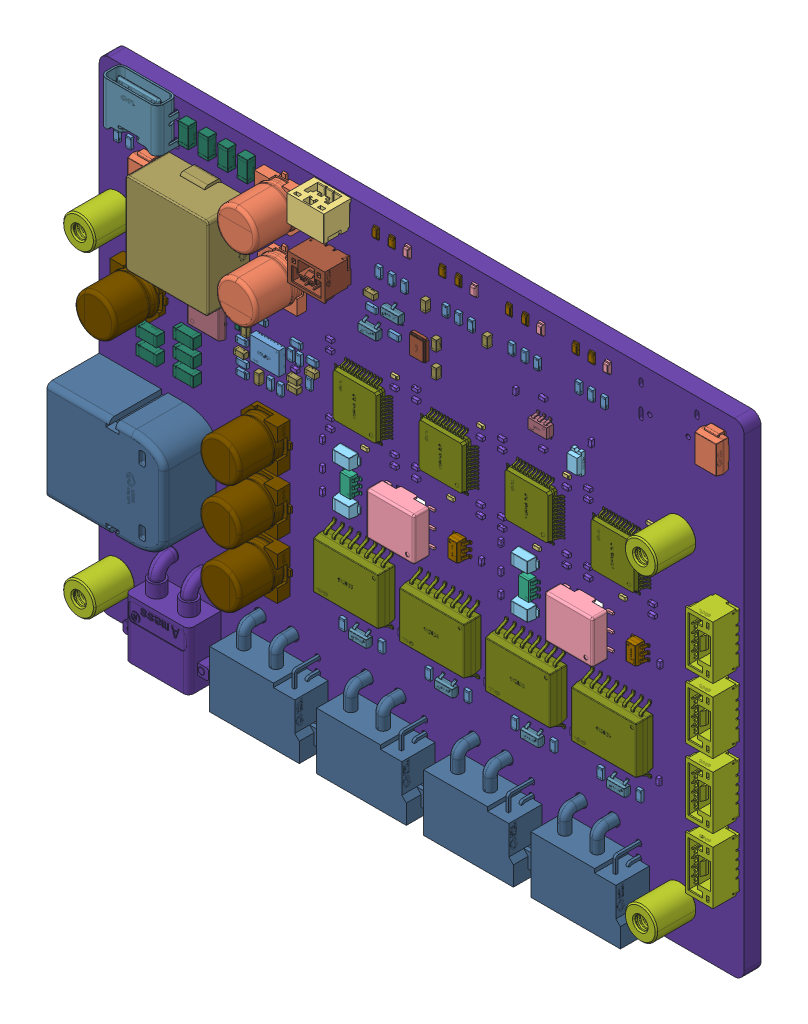
SolidWorks assembly 三合一(1), configuration 默认. Lengths in mm.
Overall size (99.98 75.08 11.76).
370 component instances, 35 part files, 0 mates.
Components (placement in the parent):
- 三合一(1).step-1: 三合一(1).step [默认] at origin size (99.98 75.08 11.76)
  - R75~R0603~R0603~5cPJ.step-1: R75~R0603~R0603~5cPJ.step [默认] at (-28.5751 -8.895 -0.01) x (0 -1 0) z (0 0 -1) size (0.81 1.62 0.45)
    - R0603~R0603~Wemx.step-1: R0603~R0603~Wemx.step [默认] at origin size (0.81 1.62 0.45)
  - R159~R0603~R0603~W8s1.step-1: R159~R0603~R0603~W8s1.step [默认] at (-17.4062 29.8554 2.6401) x (-1 0 0) z (0 0 1) size (0.81 1.62 0.45)
    - R0603~R0603~Wemx.step-1: R0603~R0603~Wemx.step [默认] at origin size (0.81 1.62 0.45)
  - R160~R0603~R0603~Jkel.step-1: R160~R0603~R0603~Jkel.step [默认] at (-15.4326 29.8554 2.6401) x (-1 0 0) z (0 0 1) size (0.81 1.62 0.45)
    - R0603~R0603~Wemx.step-1: R0603~R0603~Wemx.step [默认] at origin size (0.81 1.62 0.45)
  - R164~R0603~R0603~qJS6.step-1: R164~R0603~R0603~qJS6.step [默认] at (-13.459 29.8554 2.6401) x (-1 0 0) z (0 0 1) size (0.81 1.62 0.45)
    - R0603~R0603~Wemx.step-1: R0603~R0603~Wemx.step [默认] at origin size (0.81 1.62 0.45)
  - R165~R0603~R0603~esAK.step-1: R165~R0603~R0603~esAK.step [默认] at (-7.0403 29.8554 2.6401) x (-1 0 0) z (0 0 1) size (0.81 1.62 0.45)
    - R0603~R0603~Wemx.step-1: R0603~R0603~Wemx.step [默认] at origin size (0.81 1.62 0.45)
  - R166~R0603~R0603~Am0v.step-1: R166~R0603~R0603~Am0v.step [默认] at (-5.0667 29.8554 2.6401) x (-1 0 0) z (0 0 1) size (0.81 1.62 0.45)
    - R0603~R0603~Wemx.step-1: R0603~R0603~Wemx.step [默认] at origin size (0.81 1.62 0.45)
  - R167~R0603~R0603~RGyW.step-1: R167~R0603~R0603~RGyW.step [默认] at (-3.0931 29.8554 2.6401) x (-1 0 0) z (0 0 1) size (0.81 1.62 0.45)
    - R0603~R0603~Wemx.step-1: R0603~R0603~Wemx.step [默认] at origin size (0.81 1.62 0.45)
  - R168~R0603~R0603~ARsL.step-1: R168~R0603~R0603~ARsL.step [默认] at (3.1985 29.8554 2.6401) x (-1 0 0) z (0 0 1) size (0.81 1.62 0.45)
    - R0603~R0603~Wemx.step-1: R0603~R0603~Wemx.step [默认] at origin size (0.81 1.62 0.45)
  - R169~R0603~R0603~JQ4Y.step-1: R169~R0603~R0603~JQ4Y.step [默认] at (5.1721 29.8554 2.6401) x (-1 0 0) z (0 0 1) size (0.81 1.62 0.45)
    - R0603~R0603~Wemx.step-1: R0603~R0603~Wemx.step [默认] at origin size (0.81 1.62 0.45)
  - R170~R0603~R0603~c30l.step-1: R170~R0603~R0603~c30l.step [默认] at (7.1457 29.8554 2.6401) x (-1 0 0) z (0 0 1) size (0.81 1.62 0.45)
    - R0603~R0603~Wemx.step-1: R0603~R0603~Wemx.step [默认] at origin size (0.81 1.62 0.45)
  - R171~R0603~R0603~cDsC.step-1: R171~R0603~R0603~cDsC.step [默认] at (13.5643 29.8554 2.6401) x (-1 0 0) z (0 0 1) size (0.81 1.62 0.45)
    - R0603~R0603~Wemx.step-1: R0603~R0603~Wemx.step [默认] at origin size (0.81 1.62 0.45)
  - R172~R0603~R0603~ldmr.step-1: R172~R0603~R0603~ldmr.step [默认] at (15.5379 29.8554 2.6401) x (-1 0 0) z (0 0 1) size (0.81 1.62 0.45)
    - R0603~R0603~Wemx.step-1: R0603~R0603~Wemx.step [默认] at origin size (0.81 1.62 0.45)
  - R173~R0603~R0603~DBhJ.step-1: R173~R0603~R0603~DBhJ.step [默认] at (17.5115 29.8554 2.6401) x (-1 0 0) z (0 0 1) size (0.81 1.62 0.45)
    - R0603~R0603~Wemx.step-1: R0603~R0603~Wemx.step [默认] at origin size (0.81 1.62 0.45)
  - R151~R0603~R0603~Tuse.step-1: R151~R0603~R0603~Tuse.step [默认] at (-18.516 24.4061 2.6401) x (0 -1 0) z (0 0 1) size (0.81 1.62 0.45)
    - R0603~R0603~Wemx.step-1: R0603~R0603~Wemx.step [默认] at origin size (0.81 1.62 0.45)
  - R137~R0603~R0603~KOhT.step-1: R137~R0603~R0603~KOhT.step [默认] at (-22.995 -20.1855 2.6401) size (0.81 1.62 0.45)
    - R0603~R0603~Wemx.step-1: R0603~R0603~Wemx.step [默认] at origin size (0.81 1.62 0.45)
  - R152~R0603~R0603~idg1.step-1: R152~R0603~R0603~idg1.step [默认] at (-15.016 22.484 2.6401) x (0 1 0) z (0 0 1) size (0.81 1.62 0.45)
    - R0603~R0603~Wemx.step-1: R0603~R0603~Wemx.step [默认] at origin size (0.81 1.62 0.45)
  - CS6~R0603~R0603~lHR4.step-1: CS6~R0603~R0603~lHR4.step [默认] at (23.005 -20.1855 2.6401) size (0.81 1.62 0.45)
    - R0603~R0603~Wemx.step-1: R0603~R0603~Wemx.step [默认] at origin size (0.81 1.62 0.45)
  - R141~R0603~R0603~uq1I.step-1: R141~R0603~R0603~uq1I.step [默认] at (-9.6617 -20.1855 2.6401) size (0.81 1.62 0.45)
    - R0603~R0603~Wemx.step-1: R0603~R0603~Wemx.step [默认] at origin size (0.81 1.62 0.45)
  - CS5~R0603~R0603~782x.step-1: CS5~R0603~R0603~782x.step [默认] at (9.6717 -20.1855 2.6401) size (0.81 1.62 0.45)
    - R0603~R0603~Wemx.step-1: R0603~R0603~Wemx.step [默认] at origin size (0.81 1.62 0.45)
  - R144~R0603~R0603~EvhU.step-1: R144~R0603~R0603~EvhU.step [默认] at (3.6717 -20.1855 2.6401) size (0.81 1.62 0.45)
    - R0603~R0603~Wemx.step-1: R0603~R0603~Wemx.step [默认] at origin size (0.81 1.62 0.45)
  - CS7~R0603~R0603~eEbJ.step-1: CS7~R0603~R0603~eEbJ.step [默认] at (-3.6617 -20.1855 2.6401) size (0.81 1.62 0.45)
    - R0603~R0603~Wemx.step-1: R0603~R0603~Wemx.step [默认] at origin size (0.81 1.62 0.45)
  - R147~R0603~R0603~I41l.step-1: R147~R0603~R0603~I41l.step [默认] at (17.005 -20.1855 2.6401) size (0.81 1.62 0.45)
    - R0603~R0603~Wemx.step-1: R0603~R0603~Wemx.step [默认] at origin size (0.81 1.62 0.45)
  - CS8~R0603~R0603~DkA6.step-1: CS8~R0603~R0603~DkA6.step [默认] at (-16.995 -20.1855 2.6401) size (0.81 1.62 0.45)
    - R0603~R0603~Wemx.step-1: R0603~R0603~Wemx.step [默认] at origin size (0.81 1.62 0.45)
  - R1~R0402~R0603~QKKM.step-1: R1~R0402~R0603~QKKM.step [默认] at (-29.788 11.9413 2.6401) x (-1 0 0) z (0 0 1) size (0.81 1.62 0.45)
    - R0603~R0603~Wemx.step-1: R0603~R0603~Wemx.step [默认] at origin size (0.81 1.62 0.45)
  - R2~R0402~R0603~ICsz.step-1: R2~R0402~R0603~ICsz.step [默认] at (-31.0503 11.9335 2.6401) size (0.81 1.62 0.45)
    - R0603~R0603~Wemx.step-1: R0603~R0603~Wemx.step [默认] at origin size (0.81 1.62 0.45)
  - R3~R0402~R0603~sk96.step-1: R3~R0402~R0603~sk96.step [默认] at (-32.6863 6.4398 2.6401) size (0.81 1.62 0.45)
    - R0603~R0603~Wemx.step-1: R0603~R0603~Wemx.step [默认] at origin size (0.81 1.62 0.45)
  - R4~R0402~R0603~okoP.step-1: R4~R0402~R0603~okoP.step [默认] at (-38.5703 5.6081 2.6401) x (0 -1 0) z (0 0 1) size (0.81 1.62 0.45)
    - R0603~R0603~Wemx.step-1: R0603~R0603~Wemx.step [默认] at origin size (0.81 1.62 0.45)
  - R5~R0402~R0603~vXkP.step-1: R5~R0402~R0603~vXkP.step [默认] at (-34.283 6.4398 2.6401) x (-1 0 0) z (0 0 1) size (0.81 1.62 0.45)
    - R0603~R0603~Wemx.step-1: R0603~R0603~Wemx.step [默认] at origin size (0.81 1.62 0.45)
  - R6~R0402~R0603~4bc1.step-1: R6~R0402~R0603~4bc1.step [默认] at (-28.1899 9.4911 2.6401) size (0.81 1.62 0.45)
    - R0603~R0603~Wemx.step-1: R0603~R0603~Wemx.step [默认] at origin size (0.81 1.62 0.45)
  - R7~R0402~R0603~K2X5.step-1: R7~R0402~R0603~K2X5.step [默认] at (-27.7516 12.6103 2.6401) x (0 -1 0) z (0 0 1) size (0.81 1.62 0.45)
    - R0603~R0603~Wemx.step-1: R0603~R0603~Wemx.step [默认] at origin size (0.81 1.62 0.45)
  - R8~R0402~R0603~ww3o.step-1: R8~R0402~R0603~ww3o.step [默认] at (-38.5577 7.046 2.6401) x (0 1 0) z (0 0 1) size (0.81 1.62 0.45)
    - R0603~R0603~Wemx.step-1: R0603~R0603~Wemx.step [默认] at origin size (0.81 1.62 0.45)
  - R9~R0402~R0603~rL22.step-1: R9~R0402~R0603~rL22.step [默认] at (-47.1895 9.6666 -0.01) x (-1 0 0) z (0 0 -1) size (0.81 1.62 0.45)
    - R0603~R0603~Wemx.step-1: R0603~R0603~Wemx.step [默认] at origin size (0.81 1.62 0.45)
  - R10~R0402~R0603~MKr8.step-1: R10~R0402~R0603~MKr8.step [默认] at (-30.2287 13.7786 2.6401) x (0 -1 0) z (0 0 1) size (0.81 1.62 0.45)
    - R0603~R0603~Wemx.step-1: R0603~R0603~Wemx.step [默认] at origin size (0.81 1.62 0.45)
  - R11~R0402~R0603~NHCh.step-1: R11~R0402~R0603~NHCh.step [默认] at (-35.6203 16.6165 2.6401) x (0 -1 0) z (0 0 1) size (0.81 1.62 0.45)
    - R0603~R0603~Wemx.step-1: R0603~R0603~Wemx.step [默认] at origin size (0.81 1.62 0.45)
  - R12~R0402~R0603~EJ67.step-1: R12~R0402~R0603~EJ67.step [默认] at (-35.62 15.4211 2.6401) x (0 1 0) z (0 0 1) size (0.81 1.62 0.45)
    - R0603~R0603~Wemx.step-1: R0603~R0603~Wemx.step [默认] at origin size (0.81 1.62 0.45)
  - R13~R0402~R0603~bliZ.step-1: R13~R0402~R0603~bliZ.step [默认] at (-35.6223 14.1624 2.6401) x (0 -1 0) z (0 0 1) size (0.81 1.62 0.45)
    - R0603~R0603~Wemx.step-1: R0603~R0603~Wemx.step [默认] at origin size (0.81 1.62 0.45)
  - R14~R0402~R0603~ipD6.step-1: R14~R0402~R0603~ipD6.step [默认] at (-38.6391 9.9522 2.6401) x (0 -1 0) z (0 0 1) size (0.81 1.62 0.45)
    - R0603~R0603~Wemx.step-1: R0603~R0603~Wemx.step [默认] at origin size (0.81 1.62 0.45)
  - R15~R0402~R0603~8ieX.step-1: R15~R0402~R0603~8ieX.step [默认] at (-28.8291 -15.616 -0.01) x (0 1 0) z (0 0 -1) size (0.81 1.62 0.45)
    - R0603~R0603~Wemx.step-1: R0603~R0603~Wemx.step [默认] at origin size (0.81 1.62 0.45)
  - R133~R0603~R0603~qmoj.step-1: R133~R0603~R0603~qmoj.step [默认] at (-56.0797 27.9566 2.6401) x (-1 0 0) z (0 0 1) size (0.81 1.62 0.45)
    - R0603~R0603~Wemx.step-1: R0603~R0603~Wemx.step [默认] at origin size (0.81 1.62 0.45)
  - R134~R0603~R0603~4lHX.step-1: R134~R0603~R0603~4lHX.step [默认] at (-57.9847 27.9566 2.6401) x (-1 0 0) z (0 0 1) size (0.81 1.62 0.45)
    - R0603~R0603~Wemx.step-1: R0603~R0603~Wemx.step [默认] at origin size (0.81 1.62 0.45)
  - D16~SMB_L4.6-W3.6-LS5.3-BI~SMB_L4.6-W3.6-LS5.3-BI~ZBYy.step-1: D16~SMB_L4.6-W3.6-LS5.3-BI~SMB_L4.6-W3.6-LS5.3-BI~ZBYy.step [默认] at (-52.8886 25.4111 2.7301) x (0 1 0) z (0 0 1) size (5.4 3.6 2.1)
    - SMB_L4.6-W3.6-LS5.3-BI~SMB_L4.6-W3.6-LS5.3-BI~m2hS.step-1: SMB_L4.6-W3.6-LS5.3-BI~SMB_L4.6-W3.6-LS5.3-BI~m2hS.step [默认] at origin size (5.4 3.6 2.1)
  - D15~SMB_L4.6-W3.6-LS5.3-BI~SMB_L4.6-W3.6-LS5.3-BI~mUhA.step-1: D15~SMB_L4.6-W3.6-LS5.3-BI~SMB_L4.6-W3.6-LS5.3-BI~mUhA.step [默认] at (35.0521 32.5121 2.7301) x (0 -1 0) z (0 0 1) size (5.4 3.6 2.1)
    - SMB_L4.6-W3.6-LS5.3-BI~SMB_L4.6-W3.6-LS5.3-BI~m2hS.step-1: SMB_L4.6-W3.6-LS5.3-BI~SMB_L4.6-W3.6-LS5.3-BI~m2hS.step [默认] at origin size (5.4 3.6 2.1)
  - R136~R0402~R0402_L1.0-W0.5-H0.4~lcg2.step-1: R136~R0402~R0402_L1.0-W0.5-H0.4~lcg2.step [默认] at (-19.6434 5 2.6301) size (1 0.5 0.36)
    - R0402~R0402_L1.0-W0.5-H0.4~H1Nt.step-1: R0402~R0402_L1.0-W0.5-H0.4~H1Nt.step [默认] at origin size (1 0.5 0.36)
  - R135~R0402~R0402_L1.0-W0.5-H0.4~7DHQ.step-1: R135~R0402~R0402_L1.0-W0.5-H0.4~7DHQ.step [默认] at (-15 17 2.6301) x (-1 0 0) z (0 0 1) size (1 0.5 0.36)
    - R0402~R0402_L1.0-W0.5-H0.4~H1Nt.step-1: R0402~R0402_L1.0-W0.5-H0.4~H1Nt.step [默认] at origin size (1 0.5 0.36)
  - R140~R0402~R0402_L1.0-W0.5-H0.4~fAPd.step-1: R140~R0402~R0402_L1.0-W0.5-H0.4~fAPd.step [默认] at (-6.3101 5 2.6301) size (1 0.5 0.36)
    - R0402~R0402_L1.0-W0.5-H0.4~H1Nt.step-1: R0402~R0402_L1.0-W0.5-H0.4~H1Nt.step [默认] at origin size (1 0.5 0.36)
  - R139~R0402~R0402_L1.0-W0.5-H0.4~Vtb0.step-1: R139~R0402~R0402_L1.0-W0.5-H0.4~Vtb0.step [默认] at (-1.6667 17 2.6301) x (-1 0 0) z (0 0 1) size (1 0.5 0.36)
    - R0402~R0402_L1.0-W0.5-H0.4~H1Nt.step-1: R0402~R0402_L1.0-W0.5-H0.4~H1Nt.step [默认] at origin size (1 0.5 0.36)
  - R143~R0402~R0402_L1.0-W0.5-H0.4~u8e5.step-1: R143~R0402~R0402_L1.0-W0.5-H0.4~u8e5.step [默认] at (7.0233 5 2.6301) size (1 0.5 0.36)
    - R0402~R0402_L1.0-W0.5-H0.4~H1Nt.step-1: R0402~R0402_L1.0-W0.5-H0.4~H1Nt.step [默认] at origin size (1 0.5 0.36)
  - R142~R0402~R0402_L1.0-W0.5-H0.4~lItk.step-1: R142~R0402~R0402_L1.0-W0.5-H0.4~lItk.step [默认] at (11.6667 17 2.6301) x (-1 0 0) z (0 0 1) size (1 0.5 0.36)
    - R0402~R0402_L1.0-W0.5-H0.4~H1Nt.step-1: R0402~R0402_L1.0-W0.5-H0.4~H1Nt.step [默认] at origin size (1 0.5 0.36)
  - R146~R0402~R0402_L1.0-W0.5-H0.4~vA6z.step-1: R146~R0402~R0402_L1.0-W0.5-H0.4~vA6z.step [默认] at (20.3567 5 2.6301) size (1 0.5 0.36)
    - R0402~R0402_L1.0-W0.5-H0.4~H1Nt.step-1: R0402~R0402_L1.0-W0.5-H0.4~H1Nt.step [默认] at origin size (1 0.5 0.36)
  - R145~R0402~R0402_L1.0-W0.5-H0.4~Remo.step-1: R145~R0402~R0402_L1.0-W0.5-H0.4~Remo.step [默认] at (24.6191 17 2.6301) x (-1 0 0) z (0 0 1) size (1 0.5 0.36)
    - R0402~R0402_L1.0-W0.5-H0.4~H1Nt.step-1: R0402~R0402_L1.0-W0.5-H0.4~H1Nt.step [默认] at origin size (1 0.5 0.36)
  - LED18~LED0603-R-RD_GREEN~LED0603-RD_GREEN~kkZH.step-1: LED18~LED0603-R-RD_GREEN~LED0603-RD_GREEN~kkZH.step [默认] at (-13 34.7338 2.6401) x (0 -1 0) z (0 0 1) size (1.62 0.8 0.6)
    - LED0603-R-RD_GREEN~LED0603-RD_GREEN~Eb2N.step-1: LED0603-R-RD_GREEN~LED0603-RD_GREEN~Eb2N.step [默认] at origin size (1.62 0.8 0.6)
  - LED21~LED0603-R-RD_GREEN~LED0603-RD_GREEN~Mnfx.step-1: LED21~LED0603-R-RD_GREEN~LED0603-RD_GREEN~Mnfx.step [默认] at (-2.6667 34.76 2.6401) x (0 -1 0) z (0 0 1) size (1.62 0.8 0.6)
    - LED0603-R-RD_GREEN~LED0603-RD_GREEN~Eb2N.step-1: LED0603-R-RD_GREEN~LED0603-RD_GREEN~Eb2N.step [默认] at origin size (1.62 0.8 0.6)
  - LED24~LED0603-R-RD_GREEN~LED0603-RD_GREEN~tHpw.step-1: LED24~LED0603-R-RD_GREEN~LED0603-RD_GREEN~tHpw.step [默认] at (7.6667 34.7338 2.6401) x (0 -1 0) z (0 0 1) size (1.62 0.8 0.6)
    - LED0603-R-RD_GREEN~LED0603-RD_GREEN~Eb2N.step-1: LED0603-R-RD_GREEN~LED0603-RD_GREEN~Eb2N.step [默认] at origin size (1.62 0.8 0.6)
  - LED27~LED0603-R-RD_GREEN~LED0603-RD_GREEN~rwUx.step-1: LED27~LED0603-R-RD_GREEN~LED0603-RD_GREEN~rwUx.step [默认] at (18 34.7338 2.6401) x (0 -1 0) z (0 0 1) size (1.62 0.8 0.6)
    - LED0603-R-RD_GREEN~LED0603-RD_GREEN~Eb2N.step-1: LED0603-R-RD_GREEN~LED0603-RD_GREEN~Eb2N.step [默认] at origin size (1.62 0.8 0.6)
  - U107~SOD-123FL_L2.8-W1.9-LS3.7-RD~SOD-123FL_L2.8-W1.9-LS3.7-RD~TyNM.step-1: U107~SOD-123FL_L2.8-W1.9-LS3.7-RD~SOD-123FL_L2.8-W1.9-LS3.7-RD~TyNM.step [默认] at (5.4499 -3.754 2.8301) size (3.6 1.9 1.4)
    - SOD-123FL_L2.8-W1.9-LS3.7-RD~SOD-123FL_L2.8-W1.9-LS3.7-RD~L6eT.step-1: SOD-123FL_L2.8-W1.9-LS3.7-RD~SOD-123FL_L2.8-W1.9-LS3.7-RD~L6eT.step [默认] at origin size (3.6 1.9 1.4)
  - U22~SOD-123FL_L2.8-W1.9-LS3.7-RD~SOD-123FL_L2.8-W1.9-LS3.7-RD~IxVu.step-1: U22~SOD-123FL_L2.8-W1.9-LS3.7-RD~SOD-123FL_L2.8-W1.9-LS3.7-RD~IxVu.step [默认] at (5.4499 2.738 2.8301) size (3.6 1.9 1.4)
    - SOD-123FL_L2.8-W1.9-LS3.7-RD~SOD-123FL_L2.8-W1.9-LS3.7-RD~L6eT.step-1: SOD-123FL_L2.8-W1.9-LS3.7-RD~SOD-123FL_L2.8-W1.9-LS3.7-RD~L6eT.step [默认] at origin size (3.6 1.9 1.4)
  - U108~SOD-123FL_L2.8-W1.9-LS3.7-RD~SOD-123FL_L2.8-W1.9-LS3.7-RD~fh98.step-1: U108~SOD-123FL_L2.8-W1.9-LS3.7-RD~SOD-123FL_L2.8-W1.9-LS3.7-RD~fh98.step [默认] at (-22.212 -3.754 2.8301) size (3.6 1.9 1.4)
    - SOD-123FL_L2.8-W1.9-LS3.7-RD~SOD-123FL_L2.8-W1.9-LS3.7-RD~L6eT.step-1: SOD-123FL_L2.8-W1.9-LS3.7-RD~SOD-123FL_L2.8-W1.9-LS3.7-RD~L6eT.step [默认] at origin size (3.6 1.9 1.4)
  - U109~SOD-123FL_L2.8-W1.9-LS3.7-RD~SOD-123FL_L2.8-W1.9-LS3.7-RD~XY9i.step-1: U109~SOD-123FL_L2.8-W1.9-LS3.7-RD~SOD-123FL_L2.8-W1.9-LS3.7-RD~XY9i.step [默认] at (-22.212 2.738 2.8301) size (3.6 1.9 1.4)
    - SOD-123FL_L2.8-W1.9-LS3.7-RD~SOD-123FL_L2.8-W1.9-LS3.7-RD~L6eT.step-1: SOD-123FL_L2.8-W1.9-LS3.7-RD~SOD-123FL_L2.8-W1.9-LS3.7-RD~L6eT.step [默认] at origin size (3.6 1.9 1.4)
  - U24~SOT-23-5_L3.0-W1.6-P0.95-LS2.8-BR~SOT-23-5_L3.0-W1.6-P0.95-LS2.8-BR~zeFX.step-1: U24~SOT-23-5_L3.0-W1.6-P0.95-LS2.8-BR~SOT-23-5_L3.0-W1.6-P0.95-LS2.8-BR~zeFX.step [默认] at (6.0001 -0.508 3.5801) size (2.8 2.95 1.25)
    - SOT-23-5_L3.0-W1.6-P0.95-LS2.8-BR~SOT-23-5_L3.0-W1.6-P0.95-LS2.8-BR~bKoc.step-1: SOT-23-5_L3.0-W1.6-P0.95-LS2.8-BR~SOT-23-5_L3.0-W1.6-P0.95-LS2.8-BR~bKoc.step [默认] at origin size (2.8 2.95 1.25)
  - U110~SOT-23-5_L3.0-W1.6-P0.95-LS2.8-BR~SOT-23-5_L3.0-W1.6-P0.95-LS2.8-BR~mHFY.step-1: U110~SOT-23-5_L3.0-W1.6-P0.95-LS2.8-BR~SOT-23-5_L3.0-W1.6-P0.95-LS2.8-BR~mHFY.step [默认] at (-21.662 -0.508 3.5801) size (2.8 2.95 1.25)
    - SOT-23-5_L3.0-W1.6-P0.95-LS2.8-BR~SOT-23-5_L3.0-W1.6-P0.95-LS2.8-BR~bKoc.step-1: SOT-23-5_L3.0-W1.6-P0.95-LS2.8-BR~SOT-23-5_L3.0-W1.6-P0.95-LS2.8-BR~bKoc.step [默认] at origin size (2.8 2.95 1.25)
  - U7~SMD_BD5.0-D3.0~SMD_BD5.0-D3.0~2Aaa.step-1: U7~SMD_BD5.0-D3.0~SMD_BD5.0-D3.0~2Aaa.step [默认] at (-57.9392 17.87 1.2301) size (5 5 7.7)
    - SMD_BD5.0-D3.0~SMD_BD5.0-D3.0~7cq1.step-1: SMD_BD5.0-D3.0~SMD_BD5.0-D3.0~7cq1.step [默认] at origin size (5 5 7.7)
  - U8~SMD_BD5.0-D3.0~SMD_BD5.0-D3.0~8QZh.step-1: U8~SMD_BD5.0-D3.0~SMD_BD5.0-D3.0~8QZh.step [默认] at (29.1449 17.87 1.2301) size (5 5 7.7)
    - SMD_BD5.0-D3.0~SMD_BD5.0-D3.0~7cq1.step-1: SMD_BD5.0-D3.0~SMD_BD5.0-D3.0~7cq1.step [默认] at origin size (5 5 7.7)
  - U9~SMD_BD5.0-D3.0~SMD_BD5.0-D3.0~xbzc.step-1: U9~SMD_BD5.0-D3.0~SMD_BD5.0-D3.0~xbzc.step [默认] at (-57.9392 -31.3381 1.2301) size (5 5 7.7)
    - SMD_BD5.0-D3.0~SMD_BD5.0-D3.0~7cq1.step-1: SMD_BD5.0-D3.0~SMD_BD5.0-D3.0~7cq1.step [默认] at origin size (5 5 7.7)
  - U10~SMD_BD5.0-D3.0~SMD_BD5.0-D3.0~ye2g.step-1: U10~SMD_BD5.0-D3.0~SMD_BD5.0-D3.0~ye2g.step [默认] at (29.1449 -31.3381 1.2301) size (5 5 7.7)
    - SMD_BD5.0-D3.0~SMD_BD5.0-D3.0~7cq1.step-1: SMD_BD5.0-D3.0~SMD_BD5.0-D3.0~7cq1.step [默认] at origin size (5 5 7.7)
  - C101~C0402~C0402_L1.0-W0.5-H0.5~urRw.step-1: C101~C0402~C0402_L1.0-W0.5-H0.5~urRw.step [默认] at (-25.0001 5 2.8801) size (1 0.5 0.5)
    - C0402~C0402_L1.0-W0.5-H0.5~4pzL.step-1: C0402~C0402_L1.0-W0.5-H0.5~4pzL.step [默认] at origin size (1 0.5 0.5)
  - C99~C0402~C0402_L1.0-W0.5-H0.5~I8ek.step-1: C99~C0402~C0402_L1.0-W0.5-H0.5~I8ek.step [默认] at (-25.0001 15.5 2.8801) size (1 0.5 0.5)
    - C0402~C0402_L1.0-W0.5-H0.5~4pzL.step-1: C0402~C0402_L1.0-W0.5-H0.5~4pzL.step [默认] at origin size (1 0.5 0.5)
  - C98~C0402~C0402_L1.0-W0.5-H0.5~H5nD.step-1: C98~C0402~C0402_L1.0-W0.5-H0.5~H5nD.step [默认] at (-25.0001 17 2.8801) size (1 0.5 0.5)
    - C0402~C0402_L1.0-W0.5-H0.5~4pzL.step-1: C0402~C0402_L1.0-W0.5-H0.5~4pzL.step [默认] at origin size (1 0.5 0.5)
  - C106~C0402~C0402_L1.0-W0.5-H0.5~xzp9.step-1: C106~C0402~C0402_L1.0-W0.5-H0.5~xzp9.step [默认] at (1.5 -0.889 2.8801) x (0 -1 0) z (0 0 1) size (1 0.5 0.5)
    - C0402~C0402_L1.0-W0.5-H0.5~4pzL.step-1: C0402~C0402_L1.0-W0.5-H0.5~4pzL.step [默认] at origin size (1 0.5 0.5)
  - C102~C0402~C0402_L1.0-W0.5-H0.5~4Dtv.step-1: C102~C0402~C0402_L1.0-W0.5-H0.5~4Dtv.step [默认] at (-25.0001 6.5 2.8801) size (1 0.5 0.5)
    - C0402~C0402_L1.0-W0.5-H0.5~4pzL.step-1: C0402~C0402_L1.0-W0.5-H0.5~4pzL.step [默认] at origin size (1 0.5 0.5)
  - C103~C0402~C0402_L1.0-W0.5-H0.5~w7rz.step-1: C103~C0402~C0402_L1.0-W0.5-H0.5~w7rz.step [默认] at (8.032 25.6541 2.8801) size (1 0.5 0.5)
    - C0402~C0402_L1.0-W0.5-H0.5~4pzL.step-1: C0402~C0402_L1.0-W0.5-H0.5~4pzL.step [默认] at origin size (1 0.5 0.5)
  - C117~C0402~C0402_L1.0-W0.5-H0.5~YPBa.step-1: C117~C0402~C0402_L1.0-W0.5-H0.5~YPBa.step [默认] at (-26.1621 -0.889 2.8801) x (0 -1 0) z (0 0 1) size (1 0.5 0.5)
    - C0402~C0402_L1.0-W0.5-H0.5~4pzL.step-1: C0402~C0402_L1.0-W0.5-H0.5~4pzL.step [默认] at origin size (1 0.5 0.5)
  - C96~C0402~C0402_L1.0-W0.5-H0.5~BI21.step-1: C96~C0402~C0402_L1.0-W0.5-H0.5~BI21.step [默认] at (-15 5 2.8801) x (-1 0 0) z (0 0 1) size (1 0.5 0.5)
    - C0402~C0402_L1.0-W0.5-H0.5~4pzL.step-1: C0402~C0402_L1.0-W0.5-H0.5~4pzL.step [默认] at origin size (1 0.5 0.5)
  - C97~C0402~C0402_L1.0-W0.5-H0.5~w74c.step-1: C97~C0402~C0402_L1.0-W0.5-H0.5~w74c.step [默认] at (-15 6.5 2.8801) x (-1 0 0) z (0 0 1) size (1 0.5 0.5)
    - C0402~C0402_L1.0-W0.5-H0.5~4pzL.step-1: C0402~C0402_L1.0-W0.5-H0.5~4pzL.step [默认] at origin size (1 0.5 0.5)
  - C100~C0402~C0402_L1.0-W0.5-H0.5~Xf4o.step-1: C100~C0402~C0402_L1.0-W0.5-H0.5~Xf4o.step [默认] at (-15 15.5 2.8801) size (1 0.5 0.5)
    - C0402~C0402_L1.0-W0.5-H0.5~4pzL.step-1: C0402~C0402_L1.0-W0.5-H0.5~4pzL.step [默认] at origin size (1 0.5 0.5)
  - C107~C0402~C0402_L1.0-W0.5-H0.5~nwPM.step-1: C107~C0402~C0402_L1.0-W0.5-H0.5~nwPM.step [默认] at (-14 -16.795 2.8801) x (0 -1 0) z (0 0 1) size (1 0.5 0.5)
    - C0402~C0402_L1.0-W0.5-H0.5~4pzL.step-1: C0402~C0402_L1.0-W0.5-H0.5~4pzL.step [默认] at origin size (1 0.5 0.5)
  - C110~C0402~C0402_L1.0-W0.5-H0.5~PXx6.step-1: C110~C0402~C0402_L1.0-W0.5-H0.5~PXx6.step [默认] at (-11.6667 5 2.8801) size (1 0.5 0.5)
    - C0402~C0402_L1.0-W0.5-H0.5~4pzL.step-1: C0402~C0402_L1.0-W0.5-H0.5~4pzL.step [默认] at origin size (1 0.5 0.5)
  - C111~C0402~C0402_L1.0-W0.5-H0.5~EMdY.step-1: C111~C0402~C0402_L1.0-W0.5-H0.5~EMdY.step [默认] at (-11.6667 6.5 2.8801) size (1 0.5 0.5)
    - C0402~C0402_L1.0-W0.5-H0.5~4pzL.step-1: C0402~C0402_L1.0-W0.5-H0.5~4pzL.step [默认] at origin size (1 0.5 0.5)
  - C115~C0402~C0402_L1.0-W0.5-H0.5~1ve2.step-1: C115~C0402~C0402_L1.0-W0.5-H0.5~1ve2.step [默认] at (-11.6667 17 2.8801) size (1 0.5 0.5)
    - C0402~C0402_L1.0-W0.5-H0.5~4pzL.step-1: C0402~C0402_L1.0-W0.5-H0.5~4pzL.step [默认] at origin size (1 0.5 0.5)
  - C112~C0402~C0402_L1.0-W0.5-H0.5~Gq7T.step-1: C112~C0402~C0402_L1.0-W0.5-H0.5~Gq7T.step [默认] at (-11.6667 15.5 2.8801) size (1 0.5 0.5)
    - C0402~C0402_L1.0-W0.5-H0.5~4pzL.step-1: C0402~C0402_L1.0-W0.5-H0.5~4pzL.step [默认] at origin size (1 0.5 0.5)
  - C118~C0402~C0402_L1.0-W0.5-H0.5~11sG.step-1: C118~C0402~C0402_L1.0-W0.5-H0.5~11sG.step [默认] at (-0.6667 -16.795 2.8801) x (0 -1 0) z (0 0 1) size (1 0.5 0.5)
    - C0402~C0402_L1.0-W0.5-H0.5~4pzL.step-1: C0402~C0402_L1.0-W0.5-H0.5~4pzL.step [默认] at origin size (1 0.5 0.5)
  - C113~C0402~C0402_L1.0-W0.5-H0.5~GWNV.step-1: C113~C0402~C0402_L1.0-W0.5-H0.5~GWNV.step [默认] at (-1.6667 15.5 2.8801) size (1 0.5 0.5)
    - C0402~C0402_L1.0-W0.5-H0.5~4pzL.step-1: C0402~C0402_L1.0-W0.5-H0.5~4pzL.step [默认] at origin size (1 0.5 0.5)
  - C105~C0402~C0402_L1.0-W0.5-H0.5~tJ99.step-1: C105~C0402~C0402_L1.0-W0.5-H0.5~tJ99.step [默认] at (1.5 -4.008 2.8801) x (0 1 0) z (0 0 1) size (1 0.5 0.5)
    - C0402~C0402_L1.0-W0.5-H0.5~4pzL.step-1: C0402~C0402_L1.0-W0.5-H0.5~4pzL.step [默认] at origin size (1 0.5 0.5)
  - C144~C0402~C0402_L1.0-W0.5-H0.5~se1Y.step-1: C144~C0402~C0402_L1.0-W0.5-H0.5~se1Y.step [默认] at (-1.5 -1.0211 2.8801) x (0 -1 0) z (0 0 1) size (1 0.5 0.5)
    - C0402~C0402_L1.0-W0.5-H0.5~4pzL.step-1: C0402~C0402_L1.0-W0.5-H0.5~4pzL.step [默认] at origin size (1 0.5 0.5)
  - C108~C0402~C0402_L1.0-W0.5-H0.5~UDsM.step-1: C108~C0402~C0402_L1.0-W0.5-H0.5~UDsM.step [默认] at (1.5 2.992 2.8801) x (0 -1 0) z (0 0 1) size (1 0.5 0.5)
    - C0402~C0402_L1.0-W0.5-H0.5~4pzL.step-1: C0402~C0402_L1.0-W0.5-H0.5~4pzL.step [默认] at origin size (1 0.5 0.5)
  - C114~C0402~C0402_L1.0-W0.5-H0.5~WxeI.step-1: C114~C0402~C0402_L1.0-W0.5-H0.5~WxeI.step [默认] at (-1.6667 5 2.8801) x (-1 0 0) z (0 0 1) size (1 0.5 0.5)
    - C0402~C0402_L1.0-W0.5-H0.5~4pzL.step-1: C0402~C0402_L1.0-W0.5-H0.5~4pzL.step [默认] at origin size (1 0.5 0.5)
  - C109~C0402~C0402_L1.0-W0.5-H0.5~FWu9.step-1: C109~C0402~C0402_L1.0-W0.5-H0.5~FWu9.step [默认] at (-1.6667 6.5 2.8801) x (-1 0 0) z (0 0 1) size (1 0.5 0.5)
    - C0402~C0402_L1.0-W0.5-H0.5~4pzL.step-1: C0402~C0402_L1.0-W0.5-H0.5~4pzL.step [默认] at origin size (1 0.5 0.5)
  - C116~C0402~C0402_L1.0-W0.5-H0.5~qAEU.step-1: C116~C0402~C0402_L1.0-W0.5-H0.5~qAEU.step [默认] at (-26.1621 -4.008 2.8801) x (0 1 0) z (0 0 1) size (1 0.5 0.5)
    - C0402~C0402_L1.0-W0.5-H0.5~4pzL.step-1: C0402~C0402_L1.0-W0.5-H0.5~4pzL.step [默认] at origin size (1 0.5 0.5)
  - C145~C0402~C0402_L1.0-W0.5-H0.5~hWgF.step-1: C145~C0402~C0402_L1.0-W0.5-H0.5~hWgF.step [默认] at (15.5105 23.3861 2.8801) x (0 1 0) z (0 0 1) size (1 0.5 0.5)
    - C0402~C0402_L1.0-W0.5-H0.5~4pzL.step-1: C0402~C0402_L1.0-W0.5-H0.5~4pzL.step [默认] at origin size (1 0.5 0.5)
  - C119~C0402~C0402_L1.0-W0.5-H0.5~o7qS.step-1: C119~C0402~C0402_L1.0-W0.5-H0.5~o7qS.step [默认] at (-26.1621 2.992 2.8801) x (0 -1 0) z (0 0 1) size (1 0.5 0.5)
    - C0402~C0402_L1.0-W0.5-H0.5~4pzL.step-1: C0402~C0402_L1.0-W0.5-H0.5~4pzL.step [默认] at origin size (1 0.5 0.5)
  - C123~C0402~C0402_L1.0-W0.5-H0.5~4SrT.step-1: C123~C0402~C0402_L1.0-W0.5-H0.5~4SrT.step [默认] at (1.6667 5 2.8801) size (1 0.5 0.5)
    - C0402~C0402_L1.0-W0.5-H0.5~4pzL.step-1: C0402~C0402_L1.0-W0.5-H0.5~4pzL.step [默认] at origin size (1 0.5 0.5)
  - C122~C0402~C0402_L1.0-W0.5-H0.5~K5w7.step-1: C122~C0402~C0402_L1.0-W0.5-H0.5~K5w7.step [默认] at (1.6667 6.5 2.8801) size (1 0.5 0.5)
    - C0402~C0402_L1.0-W0.5-H0.5~4pzL.step-1: C0402~C0402_L1.0-W0.5-H0.5~4pzL.step [默认] at origin size (1 0.5 0.5)
  - C120~C0402~C0402_L1.0-W0.5-H0.5~T1AC.step-1: C120~C0402~C0402_L1.0-W0.5-H0.5~T1AC.step [默认] at (1.6667 15.5 2.8801) size (1 0.5 0.5)
    - C0402~C0402_L1.0-W0.5-H0.5~4pzL.step-1: C0402~C0402_L1.0-W0.5-H0.5~4pzL.step [默认] at origin size (1 0.5 0.5)
  - C126~C0402~C0402_L1.0-W0.5-H0.5~JhXN.step-1: C126~C0402~C0402_L1.0-W0.5-H0.5~JhXN.step [默认] at (1.6667 17 2.8801) size (1 0.5 0.5)
    - C0402~C0402_L1.0-W0.5-H0.5~4pzL.step-1: C0402~C0402_L1.0-W0.5-H0.5~4pzL.step [默认] at origin size (1 0.5 0.5)
  - C121~C0402~C0402_L1.0-W0.5-H0.5~p9aX.step-1: C121~C0402~C0402_L1.0-W0.5-H0.5~p9aX.step [默认] at (11.6667 5 2.8801) x (-1 0 0) z (0 0 1) size (1 0.5 0.5)
    - C0402~C0402_L1.0-W0.5-H0.5~4pzL.step-1: C0402~C0402_L1.0-W0.5-H0.5~4pzL.step [默认] at origin size (1 0.5 0.5)
  - C124~C0402~C0402_L1.0-W0.5-H0.5~36Aa.step-1: C124~C0402~C0402_L1.0-W0.5-H0.5~36Aa.step [默认] at (11.6667 15.5 2.8801) size (1 0.5 0.5)
    - C0402~C0402_L1.0-W0.5-H0.5~4pzL.step-1: C0402~C0402_L1.0-W0.5-H0.5~4pzL.step [默认] at origin size (1 0.5 0.5)
  - C44~C0402~C0402_L1.0-W0.5-H0.5~CLqB.step-1: C44~C0402~C0402_L1.0-W0.5-H0.5~CLqB.step [默认] at (12.6667 -16.795 2.8801) x (0 -1 0) z (0 0 1) size (1 0.5 0.5)
    - C0402~C0402_L1.0-W0.5-H0.5~4pzL.step-1: C0402~C0402_L1.0-W0.5-H0.5~4pzL.step [默认] at origin size (1 0.5 0.5)
  - C125~C0402~C0402_L1.0-W0.5-H0.5~V1j7.step-1: C125~C0402~C0402_L1.0-W0.5-H0.5~V1j7.step [默认] at (11.6667 6.5 2.8801) x (-1 0 0) z (0 0 1) size (1 0.5 0.5)
    - C0402~C0402_L1.0-W0.5-H0.5~4pzL.step-1: C0402~C0402_L1.0-W0.5-H0.5~4pzL.step [默认] at origin size (1 0.5 0.5)
  - C104~C0402~C0402_L1.0-W0.5-H0.5~FroK.step-1: C104~C0402~C0402_L1.0-W0.5-H0.5~FroK.step [默认] at (8.032 18.796 2.8801) size (1 0.5 0.5)
    - C0402~C0402_L1.0-W0.5-H0.5~4pzL.step-1: C0402~C0402_L1.0-W0.5-H0.5~4pzL.step [默认] at origin size (1 0.5 0.5)
  - C127~C0402~C0402_L1.0-W0.5-H0.5~1AUR.step-1: C127~C0402~C0402_L1.0-W0.5-H0.5~1AUR.step [默认] at (15 15.5 2.8801) size (1 0.5 0.5)
    - C0402~C0402_L1.0-W0.5-H0.5~4pzL.step-1: C0402~C0402_L1.0-W0.5-H0.5~4pzL.step [默认] at origin size (1 0.5 0.5)
  - C129~C0402~C0402_L1.0-W0.5-H0.5~j5cu.step-1: C129~C0402~C0402_L1.0-W0.5-H0.5~j5cu.step [默认] at (15 5 2.8801) size (1 0.5 0.5)
    - C0402~C0402_L1.0-W0.5-H0.5~4pzL.step-1: C0402~C0402_L1.0-W0.5-H0.5~4pzL.step [默认] at origin size (1 0.5 0.5)
  - C128~C0402~C0402_L1.0-W0.5-H0.5~aOaN.step-1: C128~C0402~C0402_L1.0-W0.5-H0.5~aOaN.step [默认] at (15 6.5 2.8801) size (1 0.5 0.5)
    - C0402~C0402_L1.0-W0.5-H0.5~4pzL.step-1: C0402~C0402_L1.0-W0.5-H0.5~4pzL.step [默认] at origin size (1 0.5 0.5)
  - C132~C0402~C0402_L1.0-W0.5-H0.5~cgTs.step-1: C132~C0402~C0402_L1.0-W0.5-H0.5~cgTs.step [默认] at (15 17 2.8801) size (1 0.5 0.5)
    - C0402~C0402_L1.0-W0.5-H0.5~4pzL.step-1: C0402~C0402_L1.0-W0.5-H0.5~4pzL.step [默认] at origin size (1 0.5 0.5)
  - C146~C0402~C0402_L1.0-W0.5-H0.5~mVVR.step-1: C146~C0402~C0402_L1.0-W0.5-H0.5~mVVR.step [默认] at (26.1621 -1.0211 2.8801) x (0 1 0) z (0 0 1) size (1 0.5 0.5)
    - C0402~C0402_L1.0-W0.5-H0.5~4pzL.step-1: C0402~C0402_L1.0-W0.5-H0.5~4pzL.step [默认] at origin size (1 0.5 0.5)
  - C134~C0402~C0402_L1.0-W0.5-H0.5~vzZ3.step-1: C134~C0402~C0402_L1.0-W0.5-H0.5~vzZ3.step [默认] at (26.0001 -16.795 2.8801) x (0 -1 0) z (0 0 1) size (1 0.5 0.5)
    - C0402~C0402_L1.0-W0.5-H0.5~4pzL.step-1: C0402~C0402_L1.0-W0.5-H0.5~4pzL.step [默认] at origin size (1 0.5 0.5)
  - C147~C0402~C0402_L1.0-W0.5-H0.5~F1zl.step-1: C147~C0402~C0402_L1.0-W0.5-H0.5~F1zl.step [默认] at (3.81 24.511 2.8801) x (0 -1 0) z (0 0 1) size (1 0.5 0.5)
    - C0402~C0402_L1.0-W0.5-H0.5~4pzL.step-1: C0402~C0402_L1.0-W0.5-H0.5~4pzL.step [默认] at origin size (1 0.5 0.5)
  - C130~C0402~C0402_L1.0-W0.5-H0.5~Xh7E.step-1: C130~C0402~C0402_L1.0-W0.5-H0.5~Xh7E.step [默认] at (25.0001 5 2.8801) x (-1 0 0) z (0 0 1) size (1 0.5 0.5)
    - C0402~C0402_L1.0-W0.5-H0.5~4pzL.step-1: C0402~C0402_L1.0-W0.5-H0.5~4pzL.step [默认] at origin size (1 0.5 0.5)
  - C131~C0402~C0402_L1.0-W0.5-H0.5~N6l9.step-1: C131~C0402~C0402_L1.0-W0.5-H0.5~N6l9.step [默认] at (24.6191 15.5 2.8801) size (1 0.5 0.5)
    - C0402~C0402_L1.0-W0.5-H0.5~4pzL.step-1: C0402~C0402_L1.0-W0.5-H0.5~4pzL.step [默认] at origin size (1 0.5 0.5)
  - C133~C0402~C0402_L1.0-W0.5-H0.5~8PUh.step-1: C133~C0402~C0402_L1.0-W0.5-H0.5~8PUh.step [默认] at (25.0001 6.5 2.8801) x (-1 0 0) z (0 0 1) size (1 0.5 0.5)
    - C0402~C0402_L1.0-W0.5-H0.5~4pzL.step-1: C0402~C0402_L1.0-W0.5-H0.5~4pzL.step [默认] at origin size (1 0.5 0.5)
  - C2~C0402~C0402_L1.0-W0.5-H0.5~WdVY.step-1: C2~C0402~C0402_L1.0-W0.5-H0.5~WdVY.step [默认] at (-30.4075 10.2531 2.8801) x (-1 0 0) z (0 0 1) size (1 0.5 0.5)
    - C0402~C0402_L1.0-W0.5-H0.5~4pzL.step-1: C0402~C0402_L1.0-W0.5-H0.5~4pzL.step [默认] at origin size (1 0.5 0.5)
  - LED17~LED0603-R-RD_BLUE~LED0603-R-RD_BLUE~tnb4.step-1: LED17~LED0603-R-RD_BLUE~LED0603-R-RD_BLUE~tnb4.step [默认] at (-18 34.7469 2.6401) x (0 -1 0) z (0 0 1) size (1.62 0.81 0.41)
    - LED0603-R-RD_BLUE~LED0603-R-RD_BLUE~MIzB.step-1: LED0603-R-RD_BLUE~LED0603-R-RD_BLUE~MIzB.step [默认] at origin size (1.62 0.81 0.41)
  - LED19~LED0603-R-RD_BLUE~LED0603-R-RD_BLUE~RlJU.step-1: LED19~LED0603-R-RD_BLUE~LED0603-R-RD_BLUE~RlJU.step [默认] at (-15.5 34.7469 2.6401) x (0 -1 0) z (0 0 1) size (1.62 0.81 0.41)
    - LED0603-R-RD_BLUE~LED0603-R-RD_BLUE~MIzB.step-1: LED0603-R-RD_BLUE~LED0603-R-RD_BLUE~MIzB.step [默认] at origin size (1.62 0.81 0.41)
  - LED20~LED0603-R-RD_BLUE~LED0603-R-RD_BLUE~GG1N.step-1: LED20~LED0603-R-RD_BLUE~LED0603-R-RD_BLUE~GG1N.step [默认] at (-7.6667 34.76 2.6401) x (0 -1 0) z (0 0 1) size (1.62 0.81 0.41)
    - LED0603-R-RD_BLUE~LED0603-R-RD_BLUE~MIzB.step-1: LED0603-R-RD_BLUE~LED0603-R-RD_BLUE~MIzB.step [默认] at origin size (1.62 0.81 0.41)
  - LED22~LED0603-R-RD_BLUE~LED0603-R-RD_BLUE~FBsC.step-1: LED22~LED0603-R-RD_BLUE~LED0603-R-RD_BLUE~FBsC.step [默认] at (-5.1667 34.76 2.6401) x (0 -1 0) z (0 0 1) size (1.62 0.81 0.41)
    - LED0603-R-RD_BLUE~LED0603-R-RD_BLUE~MIzB.step-1: LED0603-R-RD_BLUE~LED0603-R-RD_BLUE~MIzB.step [默认] at origin size (1.62 0.81 0.41)
  - LED23~LED0603-R-RD_BLUE~LED0603-R-RD_BLUE~3s3m.step-1: LED23~LED0603-R-RD_BLUE~LED0603-R-RD_BLUE~3s3m.step [默认] at (2.6667 34.7338 2.6401) x (0 -1 0) z (0 0 1) size (1.62 0.81 0.41)
    - LED0603-R-RD_BLUE~LED0603-R-RD_BLUE~MIzB.step-1: LED0603-R-RD_BLUE~LED0603-R-RD_BLUE~MIzB.step [默认] at origin size (1.62 0.81 0.41)
  - LED25~LED0603-R-RD_BLUE~LED0603-R-RD_BLUE~jsUB.step-1: LED25~LED0603-R-RD_BLUE~LED0603-R-RD_BLUE~jsUB.step [默认] at (5.1667 34.7338 2.6401) x (0 -1 0) z (0 0 1) size (1.62 0.81 0.41)
    - LED0603-R-RD_BLUE~LED0603-R-RD_BLUE~MIzB.step-1: LED0603-R-RD_BLUE~LED0603-R-RD_BLUE~MIzB.step [默认] at origin size (1.62 0.81 0.41)
  - LED26~LED0603-R-RD_BLUE~LED0603-R-RD_BLUE~YhWm.step-1: LED26~LED0603-R-RD_BLUE~LED0603-R-RD_BLUE~YhWm.step [默认] at (13 34.7338 2.6401) x (0 -1 0) z (0 0 1) size (1.62 0.81 0.41)
    - LED0603-R-RD_BLUE~LED0603-R-RD_BLUE~MIzB.step-1: LED0603-R-RD_BLUE~LED0603-R-RD_BLUE~MIzB.step [默认] at origin size (1.62 0.81 0.41)
  - LED28~LED0603-R-RD_BLUE~LED0603-R-RD_BLUE~ROKN.step-1: LED28~LED0603-R-RD_BLUE~LED0603-R-RD_BLUE~ROKN.step [默认] at (15.5 34.7338 2.6401) x (0 -1 0) z (0 0 1) size (1.62 0.81 0.41)
    - LED0603-R-RD_BLUE~LED0603-R-RD_BLUE~MIzB.step-1: LED0603-R-RD_BLUE~LED0603-R-RD_BLUE~MIzB.step [默认] at origin size (1.62 0.81 0.41)
  - U2~CONN-TH_4P-XT30PW-M~CONN-TH_4P-XT30PW-M~H5wb.step-1: U2~CONN-TH_4P-XT30PW-M~CONN-TH_4P-XT30PW-M~H5wb.step [默认] at (-31.7985 -31.1737 2.6004) size (15.5 12.53 7.17)
    - CONN-TH_4P-XT30PW-M~CONN-TH_4P-XT30PW-M~Uv41.step-1: CONN-TH_4P-XT30PW-M~CONN-TH_4P-XT30PW-M~Uv41.step [默认] at origin size (15.5 12.53 7.17)
  - U3~CONN-TH_4P-XT30PW-M~CONN-TH_4P-XT30PW-M~ONgG.step-1: U3~CONN-TH_4P-XT30PW-M~CONN-TH_4P-XT30PW-M~ONgG.step [默认] at (-15.2027 -31.1737 2.6004) size (15.5 12.53 7.17)
    - CONN-TH_4P-XT30PW-M~CONN-TH_4P-XT30PW-M~Uv41.step-1: CONN-TH_4P-XT30PW-M~CONN-TH_4P-XT30PW-M~Uv41.step [默认] at origin size (15.5 12.53 7.17)
  - U5~CONN-TH_4P-XT30PW-M~CONN-TH_4P-XT30PW-M~g7yJ.step-1: U5~CONN-TH_4P-XT30PW-M~CONN-TH_4P-XT30PW-M~g7yJ.step [默认] at (1.3932 -31.1737 2.6004) size (15.5 12.53 7.17)
    - CONN-TH_4P-XT30PW-M~CONN-TH_4P-XT30PW-M~Uv41.step-1: CONN-TH_4P-XT30PW-M~CONN-TH_4P-XT30PW-M~Uv41.step [默认] at origin size (15.5 12.53 7.17)
  - U6~CONN-TH_4P-XT30PW-M~CONN-TH_4P-XT30PW-M~8BNS.step-1: U6~CONN-TH_4P-XT30PW-M~CONN-TH_4P-XT30PW-M~8BNS.step [默认] at (17.989 -31.1737 2.6004) size (15.5 12.53 7.17)
    - CONN-TH_4P-XT30PW-M~CONN-TH_4P-XT30PW-M~Uv41.step-1: CONN-TH_4P-XT30PW-M~CONN-TH_4P-XT30PW-M~Uv41.step [默认] at origin size (15.5 12.53 7.17)
